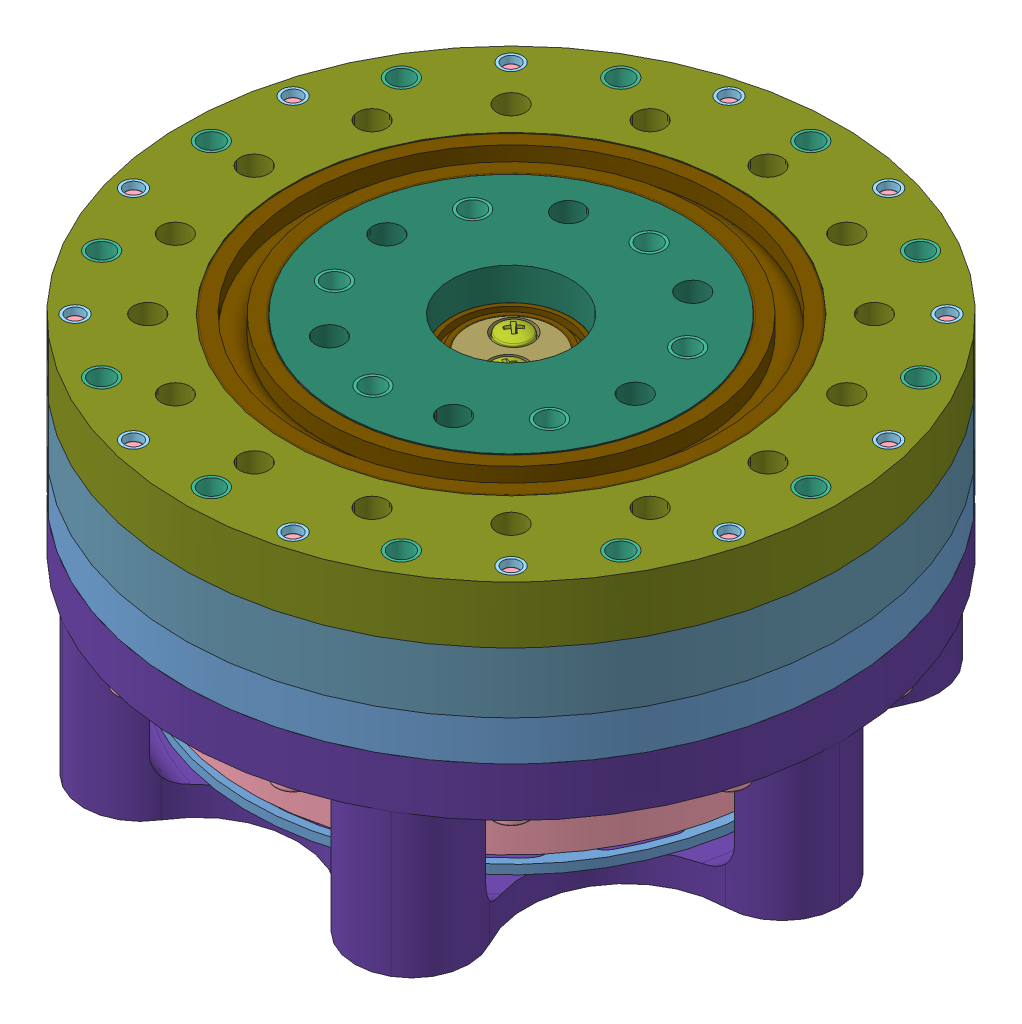
SolidWorks assembly Cycloidal, configuration Default. Lengths in mm. (continued)
Mates (geometry in assembly coordinates): (continued)
- Concentric14161: concentric aligned: cylinder of m13_bearing-11/m6-1 through (47.267 86.8573 134.1587) axis (0 1 0) radius 2; cylinder of M4x6x5.5_brass_insert-21 through (47.267 86.8573 134.1587) axis (0 1 0) radius 2
- Concentric14171: concentric aligned: cylinder of m13_bearing-1/m6-1 through (15.4472 86.8573 57.3389) axis (0 1 0) radius 2; cylinder of M4x6x5.5_brass_insert-22 through (15.4472 86.8573 57.3389) axis (0 1 0) radius 2
- Concentric14181: concentric aligned: cylinder of m13_bearing-6/m6-1 through (30.0462 86.8573 47.5841) axis (0 1 0) radius 2; cylinder of M4x6x5.5_brass_insert-23 through (30.0462 86.8573 47.5841) axis (0 1 0) radius 2
- Concentric14191: concentric aligned: cylinder of m13_bearing-12/m6-1 through (79.0868 86.8573 120.9785) axis (0 1 0) radius 2; cylinder of M4x6x5.5_brass_insert-24 through (79.0868 98.8014 120.9785) axis (0 1 0) radius 2.3
- Concentric14201: concentric aligned: cylinder of m13_bearing-5/m6-1 through (88.8416 86.8573 106.3794) axis (0 1 0) radius 2; cylinder of M4x6x5.5_brass_insert-25 through (88.8416 86.8573 106.3794) axis (0 1 0) radius 2
- Concentric14211: concentric aligned: cylinder of m13_bearing-4/m6-1 through (92.267 86.8573 89.1587) axis (0 1 0) radius 2; cylinder of M4x6x5.5_brass_insert-26 through (92.267 86.8573 89.1587) axis (0 1 0) radius 2
- Concentric14221: concentric aligned: cylinder of m13_bearing-9/m6-1 through (88.8416 86.8573 71.9379) axis (0 1 0) radius 2; cylinder of M4x6x5.5_brass_insert-27 through (88.8416 86.8573 71.9379) axis (0 1 0) radius 2
- Concentric14231: concentric aligned: line of Ring_Pin_Housing-1 through (79.0868 87.2573 57.3389) axis (0 -1 0); cylinder of M4x6x5.5_brass_insert-28 through (79.0868 92.8573 57.3389) axis (0 -1 0) radius 2
- Concentric14241: concentric aligned: cylinder of m13_bearing-7/m6-1 through (64.4877 86.8573 47.5841) axis (0 1 0) radius 2; cylinder of M4x6x5.5_brass_insert-29 through (64.4877 86.8573 47.5841) axis (0 1 0) radius 2
- Concentric14251: concentric aligned: cylinder of m13_bearing-3/m6-1 through (47.267 86.8573 44.1587) axis (0 1 0) radius 2; cylinder of M4x6x5.5_brass_insert-31 through (47.267 86.8573 44.1587) axis (0 1 0) radius 2
- Coincident1447: coincident anti-aligned: plane of m13_bearing-2/m6-1 through (64.4877 86.8573 130.7332) normal (0 1 0); plane of M4x6x5.5_brass_insert-20 through (64.4877 86.8573 130.7332) normal (0 -1 0)
- Coincident1458: coincident aligned: plane of M4x6x5.5_brass_insert-20 through (62.6232 92.8573 132.3986) normal (0 1 0); plane of M4x6x5.5_brass_insert-21 through (45.4024 92.8573 135.824) normal (0 1 0)
- Coincident1459: coincident aligned: plane of M4x6x5.5_brass_insert-20 through (62.6232 92.8573 132.3986) normal (0 1 0); plane of M4x6x5.5_brass_insert-22 through (17.0054 92.8573 59.2938) normal (0 1 0)
- Coincident1460: coincident aligned: plane of M4x6x5.5_brass_insert-20 through (62.6232 92.8573 132.3986) normal (0 1 0); plane of M4x6x5.5_brass_insert-23 through (31.6045 92.8573 49.5391) normal (0 1 0)
- Coincident1461: coincident aligned: plane of M4x6x5.5_brass_insert-20 through (62.6232 92.8573 132.3986) normal (0 1 0); plane of M4x6x5.5_brass_insert-31 through (46.7161 92.8573 46.5972) normal (0 1 0)
- Coincident1462: coincident aligned: plane of M4x6x5.5_brass_insert-20 through (62.6232 92.8573 132.3986) normal (0 1 0); plane of M4x6x5.5_brass_insert-29 through (64.1304 92.8573 50.0584) normal (0 1 0)
- Coincident1463: coincident aligned: plane of M4x6x5.5_brass_insert-20 through (62.6232 92.8573 132.3986) normal (0 1 0); plane of M4x6x5.5_brass_insert-28 through (79.0868 92.8573 57.3389) normal (0 1 0)
- Coincident1464: coincident aligned: plane of M4x6x5.5_brass_insert-20 through (62.6232 92.8573 132.3986) normal (0 1 0); plane of M4x6x5.5_brass_insert-27 through (86.977 92.8573 73.6032) normal (0 1 0)
- Coincident1465: coincident aligned: plane of M4x6x5.5_brass_insert-20 through (62.6232 92.8573 132.3986) normal (0 1 0); plane of M4x6x5.5_brass_insert-26 through (90.4024 92.8573 90.824) normal (0 1 0)
- Coincident1466: coincident aligned: plane of M4x6x5.5_brass_insert-20 through (62.6232 92.8573 132.3986) normal (0 1 0); plane of M4x6x5.5_brass_insert-25 through (86.977 92.8573 108.0448) normal (0 1 0)
- Coincident1467: coincident aligned: plane of M4x6x5.5_brass_insert-20 through (62.6232 92.8573 132.3986) normal (0 1 0); plane of M4x6x5.5_brass_insert-24 through (80.4417 92.8573 123.0795) normal (0 1 0)
- Concentric1426: concentric aligned: cylinder of pan cross head_am-1 through (44.6897 117.9573 86.0997) axis (0 1 0) radius 1.5; line of Eccentric_Shaft-1/Eccentric_Shaft_top-1 through (44.6897 90.1573 86.0997) axis (0 1 0)
- Coincident1468: coincident anti-aligned: plane of Eccentric_Shaft-1/Eccentric_Shaft_top-1 through (49.8443 90.1573 92.2177) normal (0 1 0); plane of pan cross head_am-1 through (45.6838 90.1573 84.9764) normal (0 -1 0)
- Concentric14281: concentric aligned: cylinder of pan cross head_am-3 through (49.8443 117.9573 92.2177) axis (0 1 0) radius 2.8; cylinder of Eccentric_Shaft-1/Eccentric_Shaft_top-1 through (49.8443 86.6573 92.2177) axis (0 1 0) radius 1.5
- Coincident14701: coincident anti-aligned: plane of Eccentric_Shaft-1/Eccentric_Shaft_top-1 through (44.6897 90.1573 86.0997) normal (0 1 0); plane of pan cross head_am-3 through (50.3547 90.1573 90.8072) normal (0 -1 0)
- Concentric1437: concentric anti-aligned: cylinder of Base_Plate-1 through (44.6897 76.6573 86.0997) axis (0 -1 0) radius 2; cylinder of M3x4x4.2_brass_insert-22 through (44.6897 74.5594 86.0997) axis (0 1 0) radius 1.5
- Coincident1479: coincident aligned: plane of Base_Plate-1 through (47.267 69.6573 89.1587) normal (0 -1 0); plane of M3x4x4.2_brass_insert-22 through (46.1666 69.6573 85.8375) normal (0 -1 0)
- Concentric1438: concentric anti-aligned: cylinder of Base_Plate-1 through (49.8443 76.6573 92.2177) axis (0 -1 0) radius 2; cylinder of M3x4x4.2_brass_insert-23 through (49.8443 74.5594 92.2177) axis (0 1 0) radius 1.5
- Coincident1480: coincident aligned: plane of Base_Plate-1 through (47.267 69.6573 89.1587) normal (0 -1 0); plane of M3x4x4.2_brass_insert-23 through (51.3212 69.6573 91.9555) normal (0 -1 0)
- Concentric1439: concentric anti-aligned: cylinder of Base_Plate-1 through (57.2541 76.6573 101.0123) axis (0 -1 0) radius 1.5; cylinder of pan cross head_am-4 through (57.2541 102.9573 101.0123) axis (0 1 0) radius 1.5
- Coincident1481: coincident anti-aligned: plane of Base_Plate-1 through (57.2541 75.1573 101.0123) normal (0 1 0); plane of pan cross head_am-4 through (58.7541 75.1573 101.0123) normal (0 -1 0)
- Concentric14401: concentric anti-aligned: cylinder of Base_Plate-1 through (37.2799 76.6573 77.3051) axis (0 -1 0) radius 1.5; cylinder of pan cross head_am-5 through (37.2799 102.9573 77.3051) axis (0 1 0) radius 2.8
- Coincident14821: coincident anti-aligned: plane of Base_Plate-1 through (37.2799 75.1573 77.3051) normal (0 1 0); plane of pan cross head_am-5 through (38.7799 75.1573 77.3051) normal (0 -1 0)
- Concentric144021: concentric aligned: cylinder of Cover-1 through (1.8007 97.2573 62.9087) axis (0 -1 0) radius 2.5; cylinder of M4x6x5.5_brass_insert-34 through (1.8007 85.3133 62.9087) axis (0 -1 0) radius 2.5
- Concentric144031: concentric aligned: cylinder of Cover-1 through (-5.233 97.2573 89.1587) axis (0 -1 0) radius 2.5; cylinder of M4x6x5.5_brass_insert-35 through (-5.233 97.2573 89.1587) axis (0 -1 0) radius 2
- Concentric144041: concentric aligned: cylinder of Cover-1 through (1.8007 97.2573 115.4087) axis (0 -1 0) radius 2.5; cylinder of M4x6x5.5_brass_insert-36 through (1.8007 97.2573 115.4087) axis (0 -1 0) radius 2
- Concentric144051: concentric aligned: cylinder of Cover-1 through (21.017 97.2573 134.625) axis (0 -1 0) radius 2.5; cylinder of M4x6x5.5_brass_insert-37 through (21.017 97.2573 134.625) axis (0 -1 0) radius 2
- Concentric144061: concentric aligned: cylinder of Cover-1 through (47.267 97.2573 141.6587) axis (0 -1 0) radius 2.5; cylinder of M4x6x5.5_brass_insert-38 through (47.267 97.2573 141.6587) axis (0 -1 0) radius 2
- Concentric144071: concentric aligned: cylinder of Cover-1 through (73.517 97.2573 134.625) axis (0 -1 0) radius 2.5; cylinder of M4x6x5.5_brass_insert-39 through (73.517 97.2573 134.625) axis (0 -1 0) radius 2
- Concentric144081: concentric aligned: cylinder of Cover-1 through (92.7333 97.2573 115.4087) axis (0 -1 0) radius 2.5; cylinder of M4x6x5.5_brass_insert-40 through (92.7333 97.2573 115.4087) axis (0 -1 0) radius 2
- Concentric144091: concentric aligned: cylinder of Cover-1 through (99.767 97.2573 89.1587) axis (0 -1 0) radius 2.5; cylinder of M4x6x5.5_brass_insert-41 through (99.767 97.2573 89.1587) axis (0 -1 0) radius 2
- Concentric144101: concentric aligned: cylinder of Cover-1 through (92.7333 97.2573 62.9087) axis (0 -1 0) radius 2.5; cylinder of M4x6x5.5_brass_insert-42 through (92.7333 97.2573 62.9087) axis (0 -1 0) radius 2
- Concentric144111: concentric aligned: cylinder of Cover-1 through (73.517 97.2573 43.6923) axis (0 -1 0) radius 2.5; cylinder of M4x6x5.5_brass_insert-43 through (73.517 97.2573 43.6923) axis (0 -1 0) radius 2
- Concentric144121: concentric aligned: cylinder of Cover-1 through (47.267 97.2573 36.6587) axis (0 -1 0) radius 2.5; cylinder of M4x6x5.5_brass_insert-44 through (47.267 97.2573 36.6587) axis (0 -1 0) radius 2
- Concentric144131: concentric aligned: cylinder of Cover-1 through (21.017 97.2573 43.6923) axis (0 -1 0) radius 2.5; cylinder of M4x6x5.5_brass_insert-45 through (21.017 97.2573 43.6923) axis (0 -1 0) radius 2
- Coincident14822: coincident aligned: plane of Cover-1 through (47.267 97.2573 89.1587) normal (0 1 0); plane of M4x6x5.5_brass_insert-34 through (1.8007 97.2573 62.9087) normal (0 1 0)
- Coincident14823: coincident aligned: plane of Cover-1 through (47.267 97.2573 89.1587) normal (0 1 0); plane of M4x6x5.5_brass_insert-45 through (21.017 97.2573 43.6923) normal (0 1 0)
- Coincident14824: coincident aligned: plane of Cover-1 through (47.267 97.2573 89.1587) normal (0 1 0); plane of M4x6x5.5_brass_insert-44 through (47.267 97.2573 36.6587) normal (0 1 0)
- Coincident14825: coincident aligned: plane of Cover-1 through (47.267 97.2573 89.1587) normal (0 1 0); plane of M4x6x5.5_brass_insert-43 through (73.517 97.2573 43.6923) normal (0 1 0)
- Coincident14826: coincident aligned: plane of Cover-1 through (47.267 97.2573 89.1587) normal (0 1 0); plane of M4x6x5.5_brass_insert-42 through (92.7333 97.2573 62.9087) normal (0 1 0)
- Coincident14827: coincident aligned: plane of Cover-1 through (47.267 97.2573 89.1587) normal (0 1 0); plane of M4x6x5.5_brass_insert-41 through (99.767 97.2573 89.1587) normal (0 1 0)
- Coincident14828: coincident aligned: plane of Cover-1 through (47.267 97.2573 89.1587) normal (0 1 0); plane of M4x6x5.5_brass_insert-40 through (92.7333 97.2573 115.4087) normal (0 1 0)
- Coincident14829: coincident aligned: plane of Cover-1 through (47.267 97.2573 89.1587) normal (0 1 0); plane of M4x6x5.5_brass_insert-39 through (73.517 97.2573 134.625) normal (0 1 0)
- Coincident14830: coincident aligned: plane of Cover-1 through (47.267 97.2573 89.1587) normal (0 1 0); plane of M4x6x5.5_brass_insert-38 through (47.267 97.2573 141.6587) normal (0 1 0)
- Coincident14831: coincident aligned: plane of Cover-1 through (47.267 97.2573 89.1587) normal (0 1 0); plane of M4x6x5.5_brass_insert-37 through (21.017 97.2573 134.625) normal (0 1 0)
- Coincident14832: coincident aligned: plane of Cover-1 through (47.267 97.2573 89.1587) normal (0 1 0); plane of M4x6x5.5_brass_insert-36 through (1.8007 97.2573 115.4087) normal (0 1 0)
- Coincident14833: coincident aligned: plane of Cover-1 through (47.267 97.2573 89.1587) normal (0 1 0); plane of M4x6x5.5_brass_insert-35 through (-5.233 97.2573 89.1587) normal (0 1 0)
- Concentric144161: concentric aligned: cylinder of Motor_Cover-2 through (9.0832 59.6573 50.9749) axis (0 1 0) radius 1.75; cylinder of M3x35-6 through (9.0832 132.9716 50.9749) axis (0 1 0) radius 1.5
- Concentric144171: concentric aligned: cylinder of Motor_Cover-2 through (-4.893 59.6573 75.1824) axis (0 1 0) radius 1.75; cylinder of M3x35-7 through (-4.893 132.9716 75.1824) axis (0 1 0) radius 1.5
- Concentric144181: concentric aligned: cylinder of Motor_Cover-2 through (-4.893 59.6573 103.1349) axis (0 1 0) radius 1.75; cylinder of M3x35-8 through (-4.893 132.9716 103.1349) axis (0 1 0) radius 1.5
- Concentric144191: concentric aligned: cylinder of Motor_Cover-2 through (9.0832 59.6573 127.3424) axis (0 1 0) radius 1.75; cylinder of M3x35-9 through (9.0832 132.9716 127.3424) axis (0 1 0) radius 1.5
- Concentric144201: concentric aligned: cylinder of Motor_Cover-2 through (33.2908 59.6573 141.3187) axis (0 1 0) radius 1.75; cylinder of M3x35-10 through (33.2908 132.9716 141.3187) axis (0 1 0) radius 1.5
- Concentric144211: concentric aligned: cylinder of Motor_Cover-2 through (61.2432 59.6573 141.3187) axis (0 1 0) radius 1.75; cylinder of M3x35-11 through (61.2432 132.9716 141.3187) axis (0 1 0) radius 1.5
- Concentric144221: concentric aligned: cylinder of Motor_Cover-2 through (85.4508 59.6573 127.3424) axis (0 1 0) radius 1.75; cylinder of M3x35-12 through (85.4508 132.9716 127.3424) axis (0 1 0) radius 1.5
- Concentric144231: concentric aligned: cylinder of Motor_Cover-2 through (99.427 59.6573 103.1349) axis (0 1 0) radius 1.75; cylinder of M3x35-13 through (99.427 132.9716 103.1349) axis (0 1 0) radius 1.5
- Concentric144241: concentric aligned: cylinder of Motor_Cover-2 through (99.427 59.6573 75.1824) axis (0 1 0) radius 1.75; cylinder of M3x35-14 through (99.427 132.9716 75.1824) axis (0 1 0) radius 1.5
- Concentric144251: concentric aligned: cylinder of Motor_Cover-2 through (85.4508 59.6573 50.9749) axis (0 1 0) radius 1.75; cylinder of M3x35-15 through (85.4508 132.9716 50.9749) axis (0 1 0) radius 1.5
- Concentric144261: concentric aligned: cylinder of Motor_Cover-2 through (33.2908 59.6573 36.9987) axis (0 1 0) radius 1.75; cylinder of M3x35-16 through (33.2908 132.9716 36.9987) axis (0 1 0) radius 1.5
- Concentric144271: concentric aligned: cylinder of Motor_Cover-2 through (61.2432 59.6573 36.9987) axis (0 1 0) radius 1.75; cylinder of M3x35-17 through (61.2432 132.9716 36.9987) axis (0 1 0) radius 1.5
- Coincident14836: coincident anti-aligned: plane of Motor_Cover-2 through (47.267 61.0573 34.1587) normal (0 -1 0); plane of M3x35-16 through (36.2908 61.0573 36.9987) normal (0 1 0)
- Coincident14837: coincident anti-aligned: plane of Motor_Cover-2 through (47.267 61.0573 34.1587) normal (0 -1 0); plane of M3x35-17 through (64.2432 61.0573 36.9987) normal (0 1 0)
- Coincident14838: coincident anti-aligned: plane of Motor_Cover-2 through (47.267 61.0573 34.1587) normal (0 -1 0); plane of M3x35-15 through (88.4508 61.0573 50.9749) normal (0 1 0)
- Coincident14839: coincident anti-aligned: plane of Motor_Cover-2 through (47.267 61.0573 34.1587) normal (0 -1 0); plane of M3x35-14 through (102.427 61.0573 75.1824) normal (0 1 0)
- Coincident14840: coincident anti-aligned: plane of Motor_Cover-2 through (47.267 61.0573 34.1587) normal (0 -1 0); plane of M3x35-13 through (102.427 61.0573 103.1349) normal (0 1 0)
- Coincident14841: coincident anti-aligned: plane of Motor_Cover-2 through (47.267 61.0573 34.1587) normal (0 -1 0); circle of M3x35-12
- Coincident14842: coincident anti-aligned: plane of Motor_Cover-2 through (47.267 61.0573 34.1587) normal (0 -1 0); plane of M3x35-11 through (64.2432 61.0573 141.3187) normal (0 1 0)
- Coincident14843: coincident anti-aligned: plane of Motor_Cover-2 through (47.267 61.0573 34.1587) normal (0 -1 0); plane of M3x35-10 through (36.2908 61.0573 141.3187) normal (0 1 0)
- Coincident14844: coincident anti-aligned: plane of Motor_Cover-2 through (47.267 61.0573 34.1587) normal (0 -1 0); plane of M3x35-9 through (12.0832 61.0573 127.3424) normal (0 1 0)
- Coincident14845: coincident anti-aligned: plane of Motor_Cover-2 through (47.267 61.0573 34.1587) normal (0 -1 0); plane of M3x35-8 through (-1.893 61.0573 103.1349) normal (0 1 0)
- Coincident14846: coincident anti-aligned: plane of Motor_Cover-2 through (47.267 61.0573 34.1587) normal (0 -1 0); plane of M3x35-7 through (-1.893 61.0573 75.1824) normal (0 1 0)
- Coincident14847: coincident anti-aligned: plane of Motor_Cover-2 through (47.267 61.0573 34.1587) normal (0 -1 0); plane of M3x35-6 through (12.0832 61.0573 50.9749) normal (0 1 0)
- GearMate1: gear = 10 : 1 mm: cylinder of Eccentric_Shaft-1/Eccentric_Shaft_top-1 through (47.267 91.6573 89.1587) axis (0 -1 0) radius 7.5; cylinder of Output_Shaft-1 through (47.267 97.2573 89.1587) axis (0 -1 0) radius 10.5
- Concentric1445021: concentric anti-aligned: cylinder of Base_Plate-1 through (59.1206 76.6573 79.1715) axis (0 -1 0) radius 1.5; cylinder of pan cross head_am-6 through (59.1206 102.9573 79.1715) axis (0 1 0) radius 2.8
- Coincident1486621: coincident anti-aligned: plane of Base_Plate-1 through (59.1206 75.1573 79.1715) normal (0 1 0); plane of pan cross head_am-6 through (60.6206 75.1573 79.1715) normal (0 -1 0)
- Concentric1445031: concentric anti-aligned: cylinder of Base_Plate-1 through (35.4134 76.6573 99.1458) axis (0 -1 0) radius 1.5; cylinder of pan cross head_am-7 through (35.4134 102.9573 99.1458) axis (0 1 0) radius 2.8
- Coincident1486631: coincident anti-aligned: plane of Base_Plate-1 through (35.4134 75.1573 99.1458) normal (0 1 0); plane of pan cross head_am-7 through (36.9134 75.1573 99.1458) normal (0 -1 0)
- Coincident1486632: coincident anti-aligned: plane of Cover-1 through (88.8416 86.8573 71.9379) normal (0 -1 0); plane of m13_bearing-9/radial ball bearing_68_iso-2 through (91.6245 86.8573 68.9955) normal (0 1 0)
- Coincident1486633: coincident anti-aligned: plane of Cover-1 through (88.8416 86.8573 71.9379) normal (0 -1 0); plane of m13_bearing-8/radial ball bearing_68_iso-2 through (78.4447 86.8573 53.3401) normal (0 1 0)
- Coincident1486634: coincident anti-aligned: plane of Cover-1 through (88.8416 86.8573 71.9379) normal (0 -1 0); plane of m13_bearing-7/radial ball bearing_68_iso-2 through (66.6983 86.8573 44.1906) normal (0 1 0)
- Coincident1486635: coincident anti-aligned: plane of Cover-1 through (88.8416 86.8573 71.9379) normal (0 -1 0); plane of m13_bearing-3/radial ball bearing_68_iso-2 through (47.4539 86.8573 40.113) normal (0 1 0)
- Coincident1486636: coincident anti-aligned: plane of Cover-1 through (88.8416 86.8573 71.9379) normal (0 -1 0); plane of m13_bearing-4/radial ball bearing_68_iso-2 through (92.1768 86.8573 85.1097) normal (0 1 0)
- Coincident1486637: coincident anti-aligned: plane of Cover-1 through (88.8416 86.8573 71.9379) normal (0 -1 0); plane of m13_bearing-5/radial ball bearing_68_iso-2 through (88.6021 86.8573 102.3365) normal (0 1 0)
- Coincident1486638: coincident anti-aligned: plane of Cover-1 through (88.8416 86.8573 71.9379) normal (0 -1 0); plane of m13_bearing-12/radial ball bearing_68_iso-2 through (78.3409 86.8573 116.9978) normal (0 1 0)
- Coincident1486639: coincident anti-aligned: plane of Cover-1 through (88.8416 86.8573 71.9379) normal (0 -1 0); plane of m13_bearing-11/radial ball bearing_68_iso-2 through (44.9443 86.8573 130.8409) normal (0 1 0)
- Coincident1486640: coincident anti-aligned: plane of Cover-1 through (88.8416 86.8573 71.9379) normal (0 -1 0); plane of m13_bearing-2/radial ball bearing_68_iso-2 through (64.0006 86.8573 126.7126) normal (0 1 0)
- Coincident1486643: coincident anti-aligned: plane of Cover-1 through (30.0462 86.8573 47.5841) normal (0 -1 0); plane of m13_bearing-6/radial ball bearing_68_iso-2 through (28.2174 86.8573 43.9705) normal (0 1 0)
- Coincident1486644: coincident anti-aligned: plane of Cover-1 through (15.4472 86.8573 57.3389) normal (0 -1 0); plane of m13_bearing-1/radial ball bearing_68_iso-2 through (12.4643 86.8573 54.5994) normal (0 1 0)
- Concentric1445035: concentric anti-aligned: cylinder of Eccentric_Shaft-1/Eccentric_Shaft_bot-1 through (48.4141 81.6573 88.1922) axis (0 -1 0) radius 7.5; cylinder of radial ball bearing_68_iso-46 through (48.4141 59.0198 88.1922) axis (0 1 0) radius 7.5
- Coincident1486648: coincident aligned: plane of Eccentric_Shaft-1/Eccentric_Shaft_bot-1 through (48.4141 81.6573 88.1922) normal (0 1 0); plane of radial ball bearing_68_iso-46 through (40.7141 81.6573 88.1922) normal (0 1 0)
- Concentric1445036: concentric anti-aligned: cylinder of Eccentric_Shaft-1/Eccentric_Shaft_bot-2 through (46.1199 86.6573 90.1252) axis (0 -1 0) radius 7.5; cylinder of radial ball bearing_68_iso-44 through (46.1199 64.0198 90.1252) axis (0 1 0) radius 7.5
- Coincident1486649: coincident aligned: plane of Eccentric_Shaft-1/Eccentric_Shaft_bot-2 through (46.1199 82.6573 90.1252) normal (0 1 0); circle of radial ball bearing_68_iso-44
- Concentric1445037: concentric anti-aligned: cylinder of Eccentric_Shaft-1/Eccentric_Shaft_top-1 through (47.267 91.6573 89.1587) axis (0 -1 0) radius 7.5; cylinder of radial ball bearing_68_iso-45 through (47.267 69.0198 89.1587) axis (0 1 0) radius 7.5
- Concentric1445038: concentric anti-aligned: cylinder of Base_Plate-1 through (47.267 76.6573 89.1587) axis (0 -1 0) radius 20; cylinder of radial ball bearing_68_iso-40 through (47.267 52.3198 89.1587) axis (0 1 0) radius 20
- Coincident1486651: coincident aligned: plane of Base_Plate-1 through (47.267 76.6573 89.1587) normal (0 1 0); plane of Base_plate_2-1 through (47.267 76.6573 89.1587) normal (0 1 0)
- Concentric1445039: concentric anti-aligned: cylinder of Cycloidal_Discs-2 through (48.4141 81.6573 88.1922) axis (0 -1 0) radius 10.5; cylinder of radial ball bearing_68_iso-46 through (48.4141 59.0198 88.1922) axis (0 1 0) radius 10.5
- Concentric1445040: concentric aligned: cylinder of Cycloidal_Discs-1 through (46.1199 81.6573 90.1252) axis (0 1 0) radius 10.5; cylinder of radial ball bearing_68_iso-44 through (46.1199 64.0198 90.1252) axis (0 1 0) radius 10.5
- Concentric1445041: concentric anti-aligned: cylinder of radial ball bearing_68_iso-40 through (47.267 52.3198 89.1587) axis (0 1 0) radius 26; cylinder of Base_plate_2-1 through (47.267 76.6573 89.1587) axis (0 -1 0) radius 26
- Coincident1486655: coincident anti-aligned: plane of Eccentric_Shaft-1/Eccentric_Shaft_top-1 through (47.267 87.6573 89.1587) normal (0 1 0); plane of radial ball bearing_68_iso-45 through (47.5372 87.6573 97.5543) normal (0 -1 0)
- Concentric1445042: concentric anti-aligned: cylinder of Base_Plate-1 through (49.8443 76.6573 92.2177) axis (0 -1 0) radius 2; cylinder of Eccentric_Shaft-1/Eccentric_Shaft_bot-1 through (49.8443 76.6573 92.2177) axis (0 1 0) radius 1.5
- Concentric1445043: concentric aligned: cylinder of Eccentric_Shaft-1/Eccentric_Shaft_bot-1 through (44.6897 76.6573 86.0997) axis (0 1 0) radius 1.5; cylinder of M3x4x4.2_brass_insert-22 through (44.6897 74.5594 86.0997) axis (0 1 0) radius 1.5
- Concentric1445044: concentric aligned: cylinder of Base_plate_2-1 through (79.0868 76.6573 57.3389) axis (0 -1 0) radius 2.5; cylinder of socket button head screw_iso-37 through (79.0868 67.4573 57.3389) axis (0 -1 0) radius 2
- Coincident1486656: coincident anti-aligned: plane of Base_plate_2-1 through (47.267 69.6573 89.1587) normal (0 -1 0); plane of socket button head screw_iso-37 through (77.6783 69.6573 55.9189) normal (0 1 0)
- Concentric1445045: concentric aligned: cylinder of Base_plate_2-1 through (64.4877 76.6573 130.7332) axis (0 -1 0) radius 2.5; cylinder of socket button head screw_iso-38 through (64.4877 67.4573 130.7332) axis (0 -1 0) radius 2
- Coincident1486657: coincident anti-aligned: plane of Base_plate_2-1 through (47.267 69.6573 89.1587) normal (0 -1 0); plane of socket button head screw_iso-38 through (63.1085 69.6573 129.285) normal (0 1 0)
- Coincident1486658: coincident aligned: plane of Cycloidal_Discs-1 through (47.0836 86.6573 128.4748) normal (0 1 0); plane of radial ball bearing_68_iso-44 through (53.3213 86.6573 82.7612) normal (0 1 0)
- Coincident1486659: coincident aligned: plane of Cycloidal_Discs-2 through (56.2384 81.6573 50.6368) normal (0 1 0); plane of radial ball bearing_68_iso-46 through (38.1141 81.6573 88.1922) normal (0 1 0)
- Coincident1486660: coincident aligned: plane of Cover-1 through (5.6924 86.8573 71.9379) normal (0 -1 0); circle of m13_bearing-31/radial ball bearing_68_iso-2
- Coincident1486661: coincident aligned: plane of Cover-1 through (5.6924 86.8573 71.9379) normal (0 -1 0); circle of m13_bearing-32/radial ball bearing_68_iso-2
- Coincident1486662: coincident aligned: plane of Cover-1 through (5.6924 86.8573 71.9379) normal (0 -1 0); circle of m13_bearing-36/radial ball bearing_68_iso-2
- Coincident1486663: coincident aligned: plane of Cover-1 through (5.6924 86.8573 71.9379) normal (0 -1 0); circle of m13_bearing-35/radial ball bearing_68_iso-2
- Coincident1486664: coincident aligned: plane of Cover-1 through (5.6924 86.8573 71.9379) normal (0 -1 0); circle of m13_bearing-34/radial ball bearing_68_iso-2
- Concentric1445052: concentric aligned: circle of m13_bearing-31/m6-1; cylinder of M4x6x5.5_brass_insert-47 through (5.6924 92.8573 71.9379) axis (0 -1 0) radius 2
- Concentric14450531: concentric aligned: line of Cover-1 through (5.6924 86.8573 106.3794) axis (0 1 0); cylinder of M4x6x5.5_brass_insert-49 through (5.6924 87.0073 106.3794) axis (0 1 0) radius 2
- Concentric14450541: concentric aligned: line of Cover-1 through (15.4472 86.8573 120.9785) axis (0 1 0); cylinder of M4x6x5.5_brass_insert-50 through (15.4472 86.8573 120.9785) axis (0 1 0) radius 2
- Concentric1445056: concentric aligned: circle of m13_bearing-32/m6-1; cylinder of M4x6x5.5_brass_insert-48 through (2.267 92.8573 89.1587) axis (0 -1 0) radius 2
- Concentric1445057: concentric aligned: cylinder of Base_plate_2-1 through (5.6924 76.6573 71.9379) axis (0 -1 0) radius 2.5; cylinder of m13_bearing-31/radial ball bearing_68_iso-2 through (5.6924 104.9948 71.9379) axis (0 -1 0) radius 6.5
- Concentric1445058: concentric aligned: cylinder of Ring_Pin_Housing-1 through (2.267 87.2573 89.1587) axis (0 -1 0) radius 7; cylinder of m13_bearing-32/radial ball bearing_68_iso-2 through (2.267 104.9948 89.1587) axis (0 -1 0) radius 6.5
- Concentric1445059: concentric aligned: cylinder of Ring_Pin_Housing-1 through (5.6924 87.2573 106.3794) axis (0 -1 0) radius 7; cylinder of m13_bearing-36/radial ball bearing_68_iso-2 through (5.6924 105.1448 106.3794) axis (0 -1 0) radius 6.5
- Concentric1445060: concentric aligned: cylinder of Ring_Pin_Housing-1 through (15.4472 87.2573 120.9785) axis (0 -1 0) radius 7; cylinder of m13_bearing-35/radial ball bearing_68_iso-2 through (15.4472 104.9948 120.9785) axis (0 -1 0) radius 6.5
- Concentric1445061: concentric aligned: cylinder of Ring_Pin_Housing-1 through (30.0462 87.2573 130.7332) axis (0 -1 0) radius 7; cylinder of m13_bearing-34/radial ball bearing_68_iso-2 through (30.0462 105.1448 130.7332) axis (0 -1 0) radius 6.5
- Coincident1486681: coincident anti-aligned: plane of m13_bearing-1/m6-1 through (15.4472 92.8573 57.3389) normal (0 1 0); circle of M4x6x5.5_brass_insert-47
- Concentric1445063: concentric aligned: cylinder of m13_bearing-34/m6-1 through (30.0462 87.0073 130.7332) axis (0 1 0) radius 2; cylinder of M4x6x5.5_brass_insert-51 through (30.0462 87.0073 130.7332) axis (0 1 0) radius 2
- Coincident1486686: coincident aligned: plane of m13_bearing-36/m6-1 through (5.6924 93.0073 106.3794) normal (0 1 0); circle of M4x6x5.5_brass_insert-49
- Coincident1486687: coincident anti-aligned: plane of m13_bearing-32/m6-1 through (2.267 92.8573 89.1587) normal (0 1 0); circle of M4x6x5.5_brass_insert-48
- Coincident1486688: coincident aligned: plane of m13_bearing-35/m6-1 through (15.4472 92.8573 120.9785) normal (0 1 0); circle of M4x6x5.5_brass_insert-50
- Coincident1486690: coincident aligned: plane of m13_bearing-34/m6-1 through (30.0462 93.0073 130.7332) normal (0 1 0); circle of M4x6x5.5_brass_insert-51
- Concentric14450542: concentric anti-aligned: circle of Motor_Cover-2; circle of foc-motor-controller.step-1/foc-motor-controller_PCB.step-1
- Concentric14450543: concentric anti-aligned: cylinder of Motor_Cover-2 through (77.6726 61.0573 89.1587) axis (0 -1 0) radius 1.5; cylinder of foc-motor-controller.step-1/foc-motor-controller_PCB.step-1 through (77.6726 33.7033 89.1587) axis (0 1 0) radius 1.6
- Coincident1486691: coincident anti-aligned: plane of Motor_Cover-2 through (47.267 36.0573 89.1587) normal (0 -1 0); plane of hex nut style 1 gradeab_iso-1 through (47.267 36.0573 61.9285) normal (0 1 0)
- Concentric14450544: concentric aligned: cylinder of Motor_Cover-2 through (47.267 61.0573 58.7531) axis (0 -1 0) radius 1.5; cylinder of hex nut style 1 gradeab_iso-1 through (47.267 36.0573 58.7531) axis (0 -1 0) radius 1.25
- Coincident1486692: coincident anti-aligned: plane of foc-motor-controller.step-1/foc-motor-controller_PCB.step-1 through (47.267 33.6573 89.1587) normal (0 1 0); plane of hex nut style 1 gradeab_iso-1 through (47.267 33.6573 61.9285) normal (0 -1 0)
